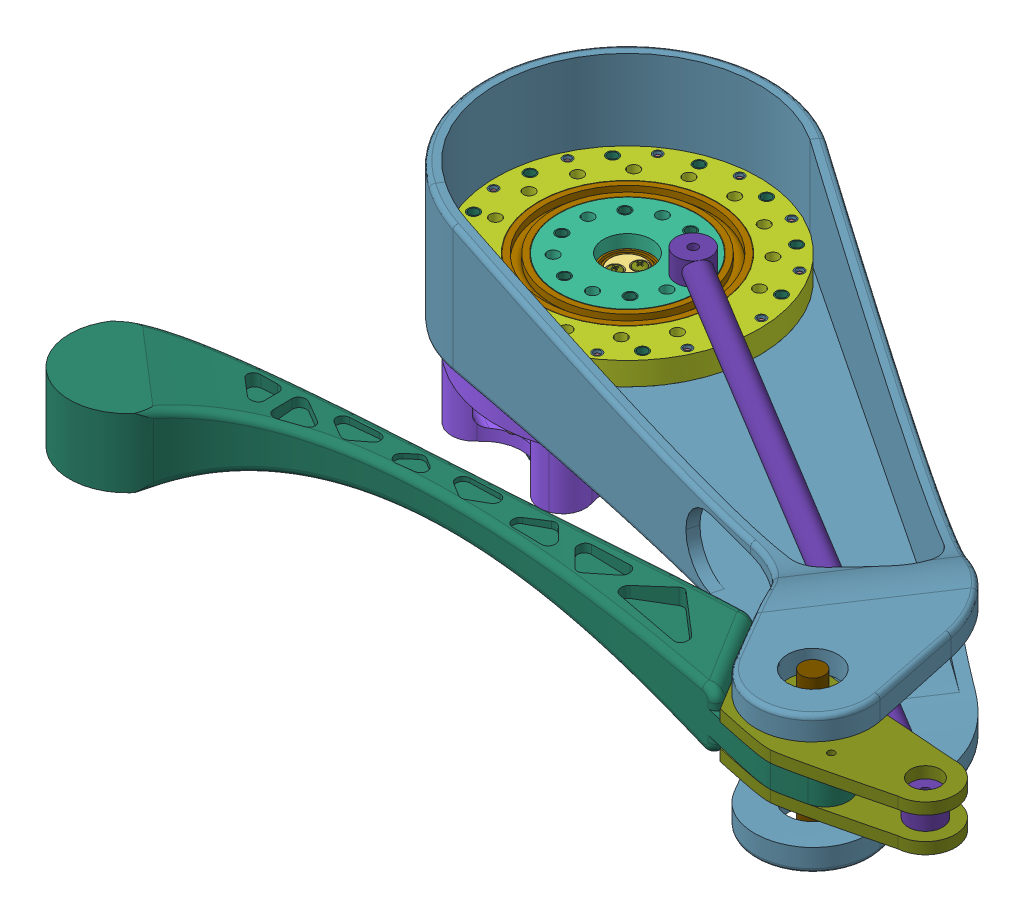
SolidWorks assembly Leg, configuration Default. Lengths in mm.
Overall size (396.87 118.19 320.81).
400 component instances, 99 part files, 9 mates.
Components (placement in the parent):
- Cycloidal-1: Cycloidal [Default] at (-40.1687 29.4235 207.1731) x (-0.342839 0 -0.939394) z (0.939394 0 -0.342839) size (162.63 70.39 162.63)
  - motor-X83008S.stp-1: motor-X83008S.stp [Default] at (19.7719 89.7915 55.1095) x (0.817868 0 0.575406) z (0 -1 0) size (114.7 114.7 37.62) (hidden)
    - base.stp-1: base.stp [Default] at (42.0794 12.0269 46.7342) size (91.6 91.6 15.61)
    - stator.stp-1: stator.stp [Default] at (42.0794 12.0269 33.1342) x (0.08493 -0.996387 0) z (0 0 1) size (83 83 8)
    - coil.stp-1: coil.stp [Default] at (39.5332 41.8984 37.1342) x (0.996387 0.08493 0) z (-0.08493 0.996387 0) size (4.4 10.2 10.5)
    - coil.stp-2: coil.stp [Default] at (34.3848 41.0025 37.1342) x (0.966502 0.256661 0) z (-0.256661 0.966502 0) size (4.4 10.2 10.5)
    - coil.stp-3: coil.stp [Default] at (29.4701 39.2261 37.1342) x (0.90725 0.420593 0) z (-0.420593 0.90725 0) size (4.4 10.2 10.5)
    - coil.stp-4: coil.stp [Default] at (24.9386 36.6233 37.1342) x (0.820431 0.571745 0) z (-0.571745 0.820431 0) size (4.4 10.2 10.5)
    - coil.stp-5: coil.stp [Default] at (20.9279 33.2732 37.1342) x (0.708685 0.705525 0) z (-0.705525 0.708685 0) size (4.4 10.2 10.5)
    - coil.stp-6: coil.stp [Default] at (17.5599 29.2775 37.1342) x (0.575405 0.817869 0) z (-0.817869 0.575405 0) size (4.4 10.2 10.5)
    - coil.stp-7: coil.stp [Default] at (14.9368 24.7576 37.1342) x (0.424642 0.905361 0) z (-0.905361 0.424642 0) size (4.4 10.2 10.5)
    - coil.stp-8: coil.stp [Default] at (13.1385 19.8509 37.1342) x (0.260976 0.965345 0) z (-0.965345 0.260976 0) size (4.4 10.2 10.5)
    - coil.stp-9: coil.stp [Default] at (12.2196 14.7066 37.1342) x (0.089381 0.995998 0) z (-0.995998 0.089381 0) size (4.4 10.2 10.5)
    - coil.stp-10: coil.stp [Default] at (12.2079 9.4807 37.1342) x (-0.08493 0.996387 0) z (-0.996387 -0.08493 0) size (4.4 10.2 10.5)
    - coil.stp-11: coil.stp [Default] at (13.1039 4.3323 37.1342) x (-0.256661 0.966502 0) z (-0.966502 -0.256661 0) size (4.4 10.2 10.5)
    - coil.stp-12: coil.stp [Default] at (14.8802 -0.5824 37.1342) x (-0.420593 0.90725 0) z (-0.90725 -0.420593 0) size (4.4 10.2 10.5)
    - coil.stp-13: coil.stp [Default] at (17.483 -5.1139 37.1342) x (-0.571745 0.820431 0) z (-0.820431 -0.571745 0) size (4.4 10.2 10.5)
    - coil.stp-14: coil.stp [Default] at (20.8332 -9.1246 37.1342) x (-0.705525 0.708685 0) z (-0.708685 -0.705525 0) size (4.4 10.2 10.5)
    - coil.stp-15: coil.stp [Default] at (24.8289 -12.4926 37.1342) x (-0.817869 0.575405 0) z (-0.575405 -0.817869 0) size (4.4 10.2 10.5)
    - coil.stp-16: coil.stp [Default] at (29.3487 -15.1157 37.1342) x (-0.905361 0.424642 0) z (-0.424642 -0.905361 0) size (4.4 10.2 10.5)
    - coil.stp-17: coil.stp [Default] at (34.2554 -16.914 37.1342) x (-0.965345 0.260976 0) z (-0.260976 -0.965345 0) size (4.4 10.2 10.5)
    - coil.stp-18: coil.stp [Default] at (39.3998 -17.8329 37.1342) x (-0.995998 0.089381 0) z (-0.089381 -0.995998 0) size (4.4 10.2 10.5)
    - coil.stp-19: coil.stp [Default] at (44.6256 -17.8446 37.1342) x (-0.996387 -0.08493 0) z (0.08493 -0.996387 0) size (4.4 10.2 10.5)
    - coil.stp-20: coil.stp [Default] at (49.7741 -16.9486 37.1342) x (-0.966502 -0.256661 0) z (0.256661 -0.966502 0) size (4.4 10.2 10.5)
    - coil.stp-21: coil.stp [Default] at (54.6887 -15.1723 37.1342) x (-0.90725 -0.420593 0) z (0.420593 -0.90725 0) size (4.4 10.2 10.5)
    - coil.stp-22: coil.stp [Default] at (59.2202 -12.5695 37.1342) x (-0.820431 -0.571745 0) z (0.571745 -0.820431 0) size (4.4 10.2 10.5)
    - coil.stp-23: coil.stp [Default] at (63.2309 -9.2193 37.1342) x (-0.708685 -0.705525 0) z (0.705525 -0.708685 0) size (4.4 10.2 10.5)
    - coil.stp-24: coil.stp [Default] at (66.599 -5.2236 37.1342) x (-0.575405 -0.817869 0) z (0.817869 -0.575405 0) size (4.4 10.2 10.5)
    - coil.stp-25: coil.stp [Default] at (69.222 -0.7038 37.1342) x (-0.424642 -0.905361 0) z (0.905361 -0.424642 0) size (4.4 10.2 10.5)
    - coil.stp-26: coil.stp [Default] at (71.0203 4.2029 37.1342) x (-0.260976 -0.965345 0) z (0.965345 -0.260976 0) size (4.4 10.2 10.5)
    - coil.stp-27: coil.stp [Default] at (71.9392 9.3473 37.1342) x (-0.089381 -0.995998 0) z (0.995998 -0.089381 0) size (4.4 10.2 10.5)
    - coil.stp-28: coil.stp [Default] at (71.9509 14.5731 37.1342) x (0.08493 -0.996387 0) z (0.996387 0.08493 0) size (4.4 10.2 10.5)
    - coil.stp-29: coil.stp [Default] at (71.055 19.7216 37.1342) x (0.256661 -0.966502 0) z (0.966502 0.256661 0) size (4.4 10.2 10.5)
    - coil.stp-30: coil.stp [Default] at (69.2786 24.6362 37.1342) x (0.420593 -0.90725 0) z (0.90725 0.420593 0) size (4.4 10.2 10.5)
    - coil.stp-31: coil.stp [Default] at (66.6758 29.1677 37.1342) x (0.571745 -0.820431 0) z (0.820431 0.571745 0) size (4.4 10.2 10.5)
    - coil.stp-32: coil.stp [Default] at (63.3257 33.1785 37.1342) x (0.705525 -0.708685 0) z (0.708685 0.705525 0) size (4.4 10.2 10.5)
    - coil.stp-33: coil.stp [Default] at (59.33 36.5465 37.1342) x (0.817869 -0.575405 0) z (0.575405 0.817869 0) size (4.4 10.2 10.5)
    - coil.stp-34: coil.stp [Default] at (54.8101 39.1695 37.1342) x (0.905361 -0.424642 0) z (0.424642 0.905361 0) size (4.4 10.2 10.5)
    - coil.stp-35: coil.stp [Default] at (49.9034 40.9678 37.1342) x (0.965345 -0.260976 0) z (0.260976 0.965345 0) size (4.4 10.2 10.5)
    - coil.stp-36: coil.stp [Default] at (44.759 41.8868 37.1342) x (0.995998 -0.089381 0) z (0.089381 0.995998 0) size (4.4 10.2 10.5)
    - rotor.stp-1: rotor.stp [Default] at (42.0794 12.0269 42.1342) x (-0.293442 0.955977 0) z (0 0 -1) size (91.8 91.8 12)
    - outrunner.stp-1: outrunner.stp [Default] at (42.0794 12.0269 30.1342) x (-0.254711 0.967017 0) z (-0.967017 -0.254711 0) size (91.8 17.01 91.8)
    - screw-mount.stp-1: screw-mount.stp [Default] at (38.1314 27.0157 27.1342) x (1 0 0) z (0 0 -1) size (7 7 6.5)
    - screw-mount.stp-2: screw-mount.stp [Default] at (27.0906 8.0789 27.1342) x (1 0 0) z (0 0 -1) size (7 7 6.5)
    - screw-mount.stp-3: screw-mount.stp [Default] at (57.0682 15.9749 27.1342) x (1 0 0) z (0 0 -1) size (7 7 6.5)
    - screw-mount.stp-4: screw-mount.stp [Default] at (46.0274 -2.9618 27.1342) x (1 0 0) z (0 0 -1) size (7 7 6.5)
    - 6702ZZ-bearing-15x21x4.stp-1: 6702ZZ-bearing-15x21x4.stp [Default] at (42.0794 12.0269 43.7342) x (1 0 0) z (0 -1 0) size (21 4 21)
    - 6702ZZ-bearing-15x21x4.stp-2: 6702ZZ-bearing-15x21x4.stp [Default] at (42.0794 12.0269 35.1342) x (1 0 0) z (0 1 0) size (21 4 21)
    - shaft.stp-1: shaft.stp [Default] at (42.0794 12.0269 20.1342) size (16 16 31.6)
    - fix-screw.stp-1: fix-screw.stp [Default] at (42.0794 12.0269 51.7342) x (1 0 0) z (0 0 -1) size (19.67 18.96 12.02)
  - Base_Plate-1: Base_Plate [Default] at (47.267 69.6573 89.1587) x (-0.64433 0 -0.764747) z (0.764747 0 -0.64433) size (40 7 40)
  - Eccentric_Shaft-1: Eccentric_Shaft [Default] at (62.181 70.3165 95.0179) x (-0.764747 0 0.64433) z (-0.64433 0 -0.764747) size (20 15 17)
    - Eccentric_Shaft_bot-1: Eccentric_Shaft_bot [Default] at (7.6302 6.3409 14.0904) size (17 5 17)
    - Eccentric_Shaft_bot-2: Eccentric_Shaft_bot [Default] at (7.6302 11.3409 14.0904) x (-1 0 0) z (0 0 -1) size (17 5 17)
    - Eccentric_Shaft_top-1: Eccentric_Shaft_top [Default] at (7.6302 16.3409 14.0904) x (-1 0 0) z (0 0 -1) size (17 5 17)
  - Cycloidal_Discs-1: Cycloidal_Discs [Default] at (46.1199 86.6573 90.1252) x (0.999784 0 -0.020763) z (-0.020763 0 -0.999784) size (79.25 5 79.73)
  - Cycloidal_Discs-2: Cycloidal_Discs [Default] at (48.4141 76.6573 88.1922) x (0.979859 0 0.19969) z (-0.19969 0 0.979859) size (79.25 5 79.73)
  - Ring_Pin_Housing-1: Ring_Pin_Housing [Default] at (47.267 76.6573 89.1587) x (0.707107 0 -0.707107) z (0.707107 0 0.707107) size (115 10.6 115)
  - Output_Shaft-1: Output_Shaft [Default] at (47.267 87.2573 89.1587) x (-0.998587 0 -0.053142) z (0.053142 0 -0.998587) size (60 10 60)
  - Cover-1: Cover [Default] at (47.267 87.2573 89.1587) x (0.707107 0 -0.707107) z (0.707107 0 0.707107) size (115 10.4 115)
  - Motor_Cover-2: Motor_Cover [Default] at (47.267 36.0573 89.1587) size (115 33.6 115)
  - radial ball bearing_68_iso-39: radial ball bearing_68_iso [ISO 15 RBB - 1860 - 32,SI,NC,32_68] at (47.267 92.2573 89.1587) x (0 1 0) z (0 0 1) size (10 78 78)
  - radial ball bearing_68_iso-40: radial ball bearing_68_iso [ISO 15 RBB - 1840 - 32,SI,NC,32_68] at (47.267 72.9573 89.1587) x (0 1 0) z (0.001003 0 0.999999) size (7 52 52)
  - Base_plate_2-1: Base_plate_2 [Default] at (47.267 69.6573 89.1587) x (0.707107 0 -0.707107) z (0.707107 0 0.707107) size (115 7 115)
  - m13_bearing-31: m13_bearing [Default] at (-10.7414 95.4081 67.0593) x (0.227678 0 0.973736) z (0.973736 0 -0.227678) size (13 16 13)
    - m6-1: m6 [Default] at (8.4921 2.5508 14.8914) size (6 16 6)
    - radial ball bearing_68_iso-1: radial ball bearing_68_iso [ISO 15 RBB - 286 - 10,SI,NC,10_68] at (8.4921 16.0508 14.8914) x (0 1 0) z (0 0 1) size (5 13 13)
    - radial ball bearing_68_iso-2: radial ball bearing_68_iso [ISO 15 RBB - 286 - 10,SI,NC,10_68] at (8.4921 11.0508 14.8914) x (0 1 0) z (0 0 1) size (5 13 13)
  - m13_bearing-32: m13_bearing [Default] at (-14.1668 95.4081 84.2801) x (0.227678 0 0.973736) z (0.973736 0 -0.227678) size (13 16 13)
    - m6-1: m6 [Default] at (8.4921 2.5508 14.8914) size (6 16 6)
    - radial ball bearing_68_iso-1: radial ball bearing_68_iso [ISO 15 RBB - 286 - 10,SI,NC,10_68] at (8.4921 16.0508 14.8914) x (0 1 0) z (0 0 1) size (5 13 13)
    - radial ball bearing_68_iso-2: radial ball bearing_68_iso [ISO 15 RBB - 286 - 10,SI,NC,10_68] at (8.4921 11.0508 14.8914) x (0 1 0) z (0 0 1) size (5 13 13)
  - m13_bearing-34: m13_bearing [Default] at (13.6125 95.5581 125.8547) x (0.227678 0 0.973736) z (0.973736 0 -0.227678) size (13 16 13)
    - m6-1: m6 [Default] at (8.4921 2.5508 14.8914) size (6 16 6)
    - radial ball bearing_68_iso-1: radial ball bearing_68_iso [ISO 15 RBB - 286 - 10,SI,NC,10_68] at (8.4921 16.0508 14.8914) x (0 1 0) z (0 0 1) size (5 13 13)
    - radial ball bearing_68_iso-2: radial ball bearing_68_iso [ISO 15 RBB - 286 - 10,SI,NC,10_68] at (8.4921 11.0508 14.8914) x (0 1 0) z (0 0 1) size (5 13 13)
  - m13_bearing-35: m13_bearing [Default] at (-0.9866 95.4081 116.0999) x (0.227678 0 0.973736) z (0.973736 0 -0.227678) size (13 16 13)
    - m6-1: m6 [Default] at (8.4921 2.5508 14.8914) size (6 16 6)
    - radial ball bearing_68_iso-1: radial ball bearing_68_iso [ISO 15 RBB - 286 - 10,SI,NC,10_68] at (8.4921 16.0508 14.8914) x (0 1 0) z (0 0 1) size (5 13 13)
    - radial ball bearing_68_iso-2: radial ball bearing_68_iso [ISO 15 RBB - 286 - 10,SI,NC,10_68] at (8.4921 11.0508 14.8914) x (0 1 0) z (0 0 1) size (5 13 13)
  - m13_bearing-36: m13_bearing [Default] at (-10.7414 95.5581 101.5009) x (0.227678 0 0.973736) z (0.973736 0 -0.227678) size (13 16 13)
    - m6-1: m6 [Default] at (8.4921 2.5508 14.8914) size (6 16 6)
    - radial ball bearing_68_iso-1: radial ball bearing_68_iso [ISO 15 RBB - 286 - 10,SI,NC,10_68] at (8.4921 16.0508 14.8914) x (0 1 0) z (0 0 1) size (5 13 13)
    - radial ball bearing_68_iso-2: radial ball bearing_68_iso [ISO 15 RBB - 286 - 10,SI,NC,10_68] at (8.4921 11.0508 14.8914) x (0 1 0) z (0 0 1) size (5 13 13)
  - m13_bearing-1: m13_bearing [Default] at (-0.8801 95.4081 62.5627) x (0.736525 0 0.676411) z (0.676411 0 -0.736525) size (13 16 13)
    - m6-1: m6 [Default] at (8.4921 2.5508 14.8914) size (6 16 6)
    - radial ball bearing_68_iso-1: radial ball bearing_68_iso [ISO 15 RBB - 286 - 10,SI,NC,10_68] at (8.4921 16.0508 14.8914) x (0 1 0) z (0 0 1) size (5 13 13)
    - radial ball bearing_68_iso-2: radial ball bearing_68_iso [ISO 15 RBB - 286 - 10,SI,NC,10_68] at (8.4921 11.0508 14.8914) x (0 1 0) z (0 0 1) size (5 13 13)
  - m13_bearing-2: m13_bearing [Default] at (48.6831 95.4081 124.0939) x (0.120271 0 0.992741) z (0.992741 0 -0.120271) size (13 16 13)
    - m6-1: m6 [Default] at (8.4921 2.5508 14.8914) size (6 16 6)
    - radial ball bearing_68_iso-1: radial ball bearing_68_iso [ISO 15 RBB - 286 - 10,SI,NC,10_68] at (8.4921 16.0508 14.8914) x (0 1 0) z (0 0 1) size (5 13 13)
    - radial ball bearing_68_iso-2: radial ball bearing_68_iso [ISO 15 RBB - 286 - 10,SI,NC,10_68] at (8.4921 11.0508 14.8914) x (0 1 0) z (0 0 1) size (5 13 13)
  - m13_bearing-3: m13_bearing [Default] at (32.7832 95.4081 34.9886) x (-0.046141 0 0.998935) z (0.998935 0 0.046141) size (13 16 13)
    - m6-1: m6 [Default] at (8.4921 2.5508 14.8914) size (6 16 6)
    - radial ball bearing_68_iso-1: radial ball bearing_68_iso [ISO 15 RBB - 286 - 10,SI,NC,10_68] at (8.4921 16.0508 14.8914) x (0 1 0) z (0 0 1) size (5 13 13)
    - radial ball bearing_68_iso-2: radial ball bearing_68_iso [ISO 15 RBB - 286 - 10,SI,NC,10_68] at (8.4921 11.0508 14.8914) x (0 1 0) z (0 0 1) size (5 13 13)
  - m13_bearing-4: m13_bearing [Default] at (77.1902 95.4081 81.0003) x (0.022268 0 0.999752) z (0.999752 0 -0.022268) size (13 16 13)
    - m6-1: m6 [Default] at (8.4921 2.5508 14.8914) size (6 16 6)
    - radial ball bearing_68_iso-1: radial ball bearing_68_iso [ISO 15 RBB - 286 - 10,SI,NC,10_68] at (8.4921 16.0508 14.8914) x (0 1 0) z (0 0 1) size (5 13 13)
    - radial ball bearing_68_iso-2: radial ball bearing_68_iso [ISO 15 RBB - 286 - 10,SI,NC,10_68] at (8.4921 11.0508 14.8914) x (0 1 0) z (0 0 1) size (5 13 13)
  - m13_bearing-5: m13_bearing [Default] at (73.474 95.4081 98.7828) x (0.059133 0 0.99825) z (0.99825 0 -0.059133) size (13 16 13)
    - m6-1: m6 [Default] at (8.4921 2.5508 14.8914) size (6 16 6)
    - radial ball bearing_68_iso-1: radial ball bearing_68_iso [ISO 15 RBB - 286 - 10,SI,NC,10_68] at (8.4921 16.0508 14.8914) x (0 1 0) z (0 0 1) size (5 13 13)
    - radial ball bearing_68_iso-2: radial ball bearing_68_iso [ISO 15 RBB - 286 - 10,SI,NC,10_68] at (8.4921 11.0508 14.8914) x (0 1 0) z (0 0 1) size (5 13 13)
  - m13_bearing-6: m13_bearing [Default] at (12.9248 95.4081 46.7315) x (0.451561 0 0.89224) z (0.89224 0 -0.451561) size (13 16 13)
    - m6-1: m6 [Default] at (8.4921 2.5508 14.8914) size (6 16 6)
    - radial ball bearing_68_iso-1: radial ball bearing_68_iso [ISO 15 RBB - 286 - 10,SI,NC,10_68] at (8.4921 16.0508 14.8914) x (0 1 0) z (0 0 1) size (5 13 13)
    - radial ball bearing_68_iso-2: radial ball bearing_68_iso [ISO 15 RBB - 286 - 10,SI,NC,10_68] at (8.4921 11.0508 14.8914) x (0 1 0) z (0 0 1) size (5 13 13)
  - m13_bearing-7: m13_bearing [Default] at (56.6452 95.4081 32.3406) x (-0.545813 0 0.837907) z (0.837907 0 0.545813) size (13 16 13)
    - m6-1: m6 [Default] at (8.4921 2.5508 14.8914) size (6 16 6)
    - radial ball bearing_68_iso-1: radial ball bearing_68_iso [ISO 15 RBB - 286 - 10,SI,NC,10_68] at (8.4921 16.0508 14.8914) x (0 1 0) z (0 0 1) size (5 13 13)
    - radial ball bearing_68_iso-2: radial ball bearing_68_iso [ISO 15 RBB - 286 - 10,SI,NC,10_68] at (8.4921 11.0508 14.8914) x (0 1 0) z (0 0 1) size (5 13 13)
  - m13_bearing-8: m13_bearing [Default] at (63.0373 95.4081 51.3153) x (0.158553 0 0.98735) z (0.98735 0 -0.158553) size (13 16 13)
    - m6-1: m6 [Default] at (8.4921 2.5508 14.8914) size (6 16 6)
    - radial ball bearing_68_iso-1: radial ball bearing_68_iso [ISO 15 RBB - 286 - 10,SI,NC,10_68] at (8.4921 16.0508 14.8914) x (0 1 0) z (0 0 1) size (5 13 13)
    - radial ball bearing_68_iso-2: radial ball bearing_68_iso [ISO 15 RBB - 286 - 10,SI,NC,10_68] at (8.4921 11.0508 14.8914) x (0 1 0) z (0 0 1) size (5 13 13)
  - m13_bearing-9: m13_bearing [Default] at (83.8577 95.4081 55.5358) x (-0.687134 0 0.72653) z (0.72653 0 0.687134) size (13 16 13)
    - m6-1: m6 [Default] at (8.4921 2.5508 14.8914) size (6 16 6)
    - radial ball bearing_68_iso-1: radial ball bearing_68_iso [ISO 15 RBB - 286 - 10,SI,NC,10_68] at (8.4921 16.0508 14.8914) x (0 1 0) z (0 0 1) size (5 13 13)
    - radial ball bearing_68_iso-2: radial ball bearing_68_iso [ISO 15 RBB - 286 - 10,SI,NC,10_68] at (8.4921 11.0508 14.8914) x (0 1 0) z (0 0 1) size (5 13 13)
  - m13_bearing-11: m13_bearing [Default] at (30.1977 95.4081 135.7424) x (0.57351 0 0.819198) z (0.819198 0 -0.57351) size (13 16 13)
    - m6-1: m6 [Default] at (8.4921 2.5508 14.8914) size (6 16 6)
    - radial ball bearing_68_iso-1: radial ball bearing_68_iso [ISO 15 RBB - 286 - 10,SI,NC,10_68] at (8.4921 16.0508 14.8914) x (0 1 0) z (0 0 1) size (5 13 13)
    - radial ball bearing_68_iso-2: radial ball bearing_68_iso [ISO 15 RBB - 286 - 10,SI,NC,10_68] at (8.4921 11.0508 14.8914) x (0 1 0) z (0 0 1) size (5 13 13)
  - m13_bearing-12: m13_bearing [Default] at (62.8861 95.4081 115.3744) x (0.184178 0 0.982893) z (0.982893 0 -0.184178) size (13 16 13)
    - m6-1: m6 [Default] at (8.4921 2.5508 14.8914) size (6 16 6)
    - radial ball bearing_68_iso-1: radial ball bearing_68_iso [ISO 15 RBB - 286 - 10,SI,NC,10_68] at (8.4921 16.0508 14.8914) x (0 1 0) z (0 0 1) size (5 13 13)
    - radial ball bearing_68_iso-2: radial ball bearing_68_iso [ISO 15 RBB - 286 - 10,SI,NC,10_68] at (8.4921 11.0508 14.8914) x (0 1 0) z (0 0 1) size (5 13 13)
  - socket button head screw_iso-2: socket button head screw_iso [ISO 7380 - M4 x 12 - 12N] at (47.267 67.4573 134.1587) x (0 1 0) z (-0.724148 0 0.689645) size (14.2 7.6 7.6)
  - socket button head screw_iso-3: socket button head screw_iso [ISO 7380 - M4 x 12 - 12N] at (15.4472 67.4573 57.3389) x (0 1 0) z (-0.724148 0 0.689645) size (14.2 7.6 7.6)
  - socket button head screw_iso-4: socket button head screw_iso [ISO 7380 - M4 x 12 - 12N] at (30.0462 67.4573 47.5841) x (0 1 0) z (-0.724148 0 0.689645) size (14.2 7.6 7.6)
  - socket button head screw_iso-5: socket button head screw_iso [ISO 7380 - M4 x 12 - 12N] at (47.267 67.4573 44.1587) x (0 1 0) z (-0.724148 0 0.689645) size (14.2 7.6 7.6)
  - socket button head screw_iso-6: socket button head screw_iso [ISO 7380 - M4 x 12 - 12N] at (64.4877 67.4573 47.5841) x (0 1 0) z (-0.724148 0 0.689645) size (14.2 7.6 7.6)
  - socket button head screw_iso-8: socket button head screw_iso [ISO 7380 - M4 x 12 - 12N] at (88.8416 67.4573 71.9379) x (0 1 0) z (-0.724148 0 0.689645) size (14.2 7.6 7.6)
  - socket button head screw_iso-9: socket button head screw_iso [ISO 7380 - M4 x 12 - 12N] at (92.267 67.4573 89.1587) x (0 1 0) z (-0.724148 0 0.689645) size (14.2 7.6 7.6)
  - socket button head screw_iso-10: socket button head screw_iso [ISO 7380 - M4 x 12 - 12N] at (88.8416 67.4573 106.3794) x (0 1 0) z (-0.724148 0 0.689645) size (14.2 7.6 7.6)
  - socket button head screw_iso-11: socket button head screw_iso [ISO 7380 - M4 x 12 - 12N] at (79.0868 67.4573 120.9785) x (0 1 0) z (-0.724148 0 0.689645) size (14.2 7.6 7.6)
  - M3x35-6: M3x35 [Default] at (9.0832 59.8573 50.9749) size (6 36.2 6)
  - M3x35-7: M3x35 [Default] at (-4.893 59.8573 75.1824) size (6 36.2 6)
  - M3x35-8: M3x35 [Default] at (-4.893 59.8573 103.1349) size (6 36.2 6)
  - M3x35-9: M3x35 [Default] at (9.0832 59.8573 127.3424) size (6 36.2 6)
  - M3x35-10: M3x35 [Default] at (33.2908 59.8573 141.3187) size (6 36.2 6)
  - M3x35-11: M3x35 [Default] at (61.2432 59.8573 141.3187) size (6 36.2 6)
  - M3x35-12: M3x35 [Default] at (85.4508 59.8573 127.3424) size (6 36.2 6)
  - M3x35-13: M3x35 [Default] at (99.427 59.8573 103.1349) size (6 36.2 6)
  - M3x35-14: M3x35 [Default] at (99.427 59.8573 75.1824) size (6 36.2 6)
  - M3x35-15: M3x35 [Default] at (85.4508 59.8573 50.9749) size (6 36.2 6)
  - M3x35-16: M3x35 [Default] at (33.2908 59.8573 36.9987) size (6 36.2 6)
  - M3x35-17: M3x35 [Default] at (61.2432 59.8573 36.9987) size (6 36.2 6)
  - m13_bearing-13: m13_bearing [Default] at (21.9503 95.0081 60.165) x (0 0 1) z (1 0 0) size (13 16 13)
    - m6-1: m6 [Default] at (8.4921 2.5508 14.8914) size (6 16 6)
    - radial ball bearing_68_iso-1: radial ball bearing_68_iso [ISO 15 RBB - 286 - 10,SI,NC,10_68] at (8.4921 16.0508 14.8914) x (0 1 0) z (0 0 1) size (5 13 13)
    - radial ball bearing_68_iso-2: radial ball bearing_68_iso [ISO 15 RBB - 286 - 10,SI,NC,10_68] at (8.4921 11.0508 14.8914) x (0 1 0) z (0 0 1) size (5 13 13)
  - m13_bearing-14: m13_bearing [Default] at (31.351 95.0081 72.3113) x (-0.995553 0 0.094199) z (0.094199 0 0.995553) size (13 16 13)
    - m6-1: m6 [Default] at (8.4921 2.5508 14.8914) size (6 16 6)
    - radial ball bearing_68_iso-1: radial ball bearing_68_iso [ISO 15 RBB - 286 - 10,SI,NC,10_68] at (8.4921 16.0508 14.8914) x (0 1 0) z (0 0 1) size (5 13 13)
    - radial ball bearing_68_iso-2: radial ball bearing_68_iso [ISO 15 RBB - 286 - 10,SI,NC,10_68] at (8.4921 11.0508 14.8914) x (0 1 0) z (0 0 1) size (5 13 13)
  - m13_bearing-15: m13_bearing [Default] at (19.8333 95.0081 99.9459) x (0 0 1) z (1 0 0) size (13 16 13)
    - m6-1: m6 [Default] at (8.4921 2.5508 14.8914) size (6 16 6)
    - radial ball bearing_68_iso-1: radial ball bearing_68_iso [ISO 15 RBB - 286 - 10,SI,NC,10_68] at (8.4921 16.0508 14.8914) x (0 1 0) z (0 0 1) size (5 13 13)
    - radial ball bearing_68_iso-2: radial ball bearing_68_iso [ISO 15 RBB - 286 - 10,SI,NC,10_68] at (8.4921 11.0508 14.8914) x (0 1 0) z (0 0 1) size (5 13 13)
  - m13_bearing-16: m13_bearing [Default] at (60.3496 95.0081 87.0135) x (0.852631 0 -0.522513) z (-0.522513 0 -0.852631) size (13 16 13)
    - m6-1: m6 [Default] at (8.4921 2.5508 14.8914) size (6 16 6)
    - radial ball bearing_68_iso-1: radial ball bearing_68_iso [ISO 15 RBB - 286 - 10,SI,NC,10_68] at (8.4921 16.0508 14.8914) x (0 1 0) z (0 0 1) size (5 13 13)
    - radial ball bearing_68_iso-2: radial ball bearing_68_iso [ISO 15 RBB - 286 - 10,SI,NC,10_68] at (8.4921 11.0508 14.8914) x (0 1 0) z (0 0 1) size (5 13 13)
  - m13_bearing-17: m13_bearing [Default] at (45.2305 95.0081 121.432) x (0.95663 0 0.291306) z (0.291306 0 -0.95663) size (13 16 13)
    - m6-1: m6 [Default] at (8.4921 2.5508 14.8914) size (6 16 6)
    - radial ball bearing_68_iso-1: radial ball bearing_68_iso [ISO 15 RBB - 286 - 10,SI,NC,10_68] at (8.4921 16.0508 14.8914) x (0 1 0) z (0 0 1) size (5 13 13)
    - radial ball bearing_68_iso-2: radial ball bearing_68_iso [ISO 15 RBB - 286 - 10,SI,NC,10_68] at (8.4921 11.0508 14.8914) x (0 1 0) z (0 0 1) size (5 13 13)
  - m13_bearing-18: m13_bearing [Default] at (55.3431 95.0081 81.8889) x (0 0 1) z (1 0 0) size (13 16 13)
    - m6-1: m6 [Default] at (8.4921 2.5508 14.8914) size (6 16 6)
    - radial ball bearing_68_iso-1: radial ball bearing_68_iso [ISO 15 RBB - 286 - 10,SI,NC,10_68] at (8.4921 16.0508 14.8914) x (0 1 0) z (0 0 1) size (5 13 13)
    - radial ball bearing_68_iso-2: radial ball bearing_68_iso [ISO 15 RBB - 286 - 10,SI,NC,10_68] at (8.4921 11.0508 14.8914) x (0 1 0) z (0 0 1) size (5 13 13)
  - M3x4x4.2_brass_insert-1: M3x4x4.2_brass_insert [Default] at (-4.893 93.2573 75.1824) x (0.984609 0 -0.174769) z (0.174769 0 0.984609) size (4 4 4)
  - M3x4x4.2_brass_insert-2: M3x4x4.2_brass_insert [Default] at (9.0832 97.2573 50.9749) x (-0.680278 0 -0.732954) z (-0.732954 0 0.680278) size (4 4 4)
  - M3x4x4.2_brass_insert-3: M3x4x4.2_brass_insert [Default] at (33.2908 97.2573 36.9987) x (-0.509546 0 -0.860444) z (-0.860444 0 0.509546) size (4 4 4)
  - M3x4x4.2_brass_insert-6: M3x4x4.2_brass_insert [Default] at (99.427 97.2573 75.1824) x (-0.680278 0 -0.732954) z (-0.732954 0 0.680278) size (4 4 4)
  - M3x4x4.2_brass_insert-8: M3x4x4.2_brass_insert [Default] at (85.4508 93.2573 127.3424) x (-0.970393 0 0.241533) z (-0.241533 0 -0.970393) size (4 4 4)
  - M3x4x4.2_brass_insert-14: M3x4x4.2_brass_insert [Default] at (61.2432 97.2573 36.9987) x (0.509546 0 0.860444) z (0.860444 0 -0.509546) size (4 4 4)
  - M3x4x4.2_brass_insert-15: M3x4x4.2_brass_insert [Default] at (85.4508 93.2573 50.9749) x (0.897191 0 -0.441644) z (0.441644 0 0.897191) size (4 4 4)
  - M3x4x4.2_brass_insert-16: M3x4x4.2_brass_insert [Default] at (99.427 97.2573 103.1349) x (-0.680278 0 -0.732954) z (-0.732954 0 0.680278) size (4 4 4)
  - M3x4x4.2_brass_insert-17: M3x4x4.2_brass_insert [Default] at (61.2432 97.2573 141.3187) x (0.680278 0 0.732954) z (0.732954 0 -0.680278) size (4 4 4)
  - M3x4x4.2_brass_insert-19: M3x4x4.2_brass_insert [Default] at (33.2908 97.2573 141.3187) x (0.680278 0 0.732954) z (0.732954 0 -0.680278) size (4 4 4)
  - M3x4x4.2_brass_insert-20: M3x4x4.2_brass_insert [Default] at (9.0832 97.2573 127.3424) x (0.680278 0 0.732954) z (0.732954 0 -0.680278) size (4 4 4)
  - M3x4x4.2_brass_insert-21: M3x4x4.2_brass_insert [Default] at (-4.893 97.2573 103.1349) x (0.680278 0 0.732954) z (0.732954 0 -0.680278) size (4 4 4)
  - M4x6x5.5_brass_insert-47: M4x6x5.5_brass_insert [Default] at (5.6924 92.8573 71.9379) x (0.474598 0 0.880203) z (0 1 0) size (5 5 6)
  - M4x6x5.5_brass_insert-48: M4x6x5.5_brass_insert [Default] at (2.267 92.8573 89.1587) x (0.260051 0 0.965595) z (0 1 0) size (5 5 6)
  - M4x6x5.5_brass_insert-49: M4x6x5.5_brass_insert [Default] at (5.6924 87.0073 106.3794) x (-0.745833 0 0.666133) z (0 -1 0) size (5 5 6)
  - M4x6x5.5_brass_insert-50: M4x6x5.5_brass_insert [Default] at (15.4472 86.8573 120.9785) x (-0.745833 0 0.666133) z (0 -1 0) size (5 5 6)
  - M4x6x5.5_brass_insert-51: M4x6x5.5_brass_insert [Default] at (30.0462 87.0073 130.7332) x (0.260051 0 -0.965595) z (0 -1 0) size (5 5 6)
  - M4x6x5.5_brass_insert-1: M4x6x5.5_brass_insert [Default] at (36.8417 86.4573 68.6571) x (-0.745833 0 0.666133) z (0 -1 0) size (5 5 6)
  - M4x6x5.5_brass_insert-4: M4x6x5.5_brass_insert [Default] at (70.2345 92.4573 90.3809) x (0.260051 0 0.965595) z (0 1 0) size (5 5 6)
  - M4x6x5.5_brass_insert-5: M4x6x5.5_brass_insert [Default] at (57.6922 92.4573 109.6602) x (0.260051 0 0.965595) z (0 1 0) size (5 5 6)
  - M4x6x5.5_brass_insert-6: M4x6x5.5_brass_insert [Default] at (34.7247 92.4573 108.438) x (0.260051 0 0.965595) z (0 1 0) size (5 5 6)
  - M4x6x5.5_brass_insert-7: M4x6x5.5_brass_insert [Default] at (24.2995 92.4573 87.9364) x (0.175665 0 0.98445) z (0 1 0) size (5 5 6)
  - M4x6x5.5_brass_insert-8: M4x6x5.5_brass_insert [Default] at (48.4892 97.2573 66.1912) x (0.260051 0 0.965595) z (0 1 0) size (5 5 6)
  - M4x6x5.5_brass_insert-9: M4x6x5.5_brass_insert [Default] at (27.9877 97.2573 76.6164) x (0.260051 0 0.965595) z (0 1 0) size (5 5 6)
  - M4x6x5.5_brass_insert-10: M4x6x5.5_brass_insert [Default] at (26.7654 97.2573 99.5839) x (0.260051 0 0.965595) z (0 1 0) size (5 5 6)
  - M4x6x5.5_brass_insert-11: M4x6x5.5_brass_insert [Default] at (46.0447 97.2573 112.1262) x (0.260051 0 0.965595) z (0 1 0) size (5 5 6)
  - M4x6x5.5_brass_insert-13: M4x6x5.5_brass_insert [Default] at (66.5463 97.2573 101.7009) x (0.260051 0 0.965595) z (0 1 0) size (5 5 6)
  - M4x6x5.5_brass_insert-14: M4x6x5.5_brass_insert [Default] at (67.7686 97.2573 78.7334) x (0.260051 0 0.965595) z (0 1 0) size (5 5 6)
  - M4x6x5.5_brass_insert-15: M4x6x5.5_brass_insert [Default] at (59.8092 92.4573 69.8794) x (0.151918 0 0.988393) z (0 1 0) size (5 5 6)
  - M4x6x5.5_brass_insert-20: M4x6x5.5_brass_insert [Default] at (64.4877 86.8573 130.7332) x (-0.745833 0 0.666133) z (0 -1 0) size (5 5 6)
  - M4x6x5.5_brass_insert-21: M4x6x5.5_brass_insert [Default] at (47.267 86.8573 134.1587) x (-0.745833 0 0.666133) z (0 -1 0) size (5 5 6)
  - M4x6x5.5_brass_insert-22: M4x6x5.5_brass_insert [Default] at (15.4472 86.8573 57.3389) x (0.623293 0 0.781988) z (0 -1 0) size (5 5 6)
  - M4x6x5.5_brass_insert-23: M4x6x5.5_brass_insert [Default] at (30.0462 86.8573 47.5841) x (0.623293 0 0.781988) z (0 -1 0) size (5 5 6)
  - M4x6x5.5_brass_insert-24: M4x6x5.5_brass_insert [Default] at (79.0868 86.8573 120.9785) x (0.541965 0 0.840401) z (0 -1 0) size (5 5 6)
  - M4x6x5.5_brass_insert-25: M4x6x5.5_brass_insert [Default] at (88.8416 86.8573 106.3794) x (-0.745833 0 0.666133) z (0 -1 0) size (5 5 6)
  - M4x6x5.5_brass_insert-26: M4x6x5.5_brass_insert [Default] at (92.267 86.8573 89.1587) x (-0.745833 0 0.666133) z (0 -1 0) size (5 5 6)
  - M4x6x5.5_brass_insert-27: M4x6x5.5_brass_insert [Default] at (88.8416 86.8573 71.9379) x (-0.745833 0 0.666133) z (0 -1 0) size (5 5 6)
  - M4x6x5.5_brass_insert-28: M4x6x5.5_brass_insert [Default] at (79.0868 92.8573 57.3389) x (0.260051 0 0.965595) z (0 1 0) size (5 5 6)
  - M4x6x5.5_brass_insert-29: M4x6x5.5_brass_insert [Default] at (64.4877 86.8573 47.5841) x (-0.142939 0 0.989731) z (0 -1 0) size (5 5 6)
  - M4x6x5.5_brass_insert-31: M4x6x5.5_brass_insert [Default] at (47.267 86.8573 44.1587) x (-0.220341 0 0.975423) z (0 -1 0) size (5 5 6)
  - M4x6x5.5_brass_insert-34: M4x6x5.5_brass_insert [Default] at (1.8007 97.2573 62.9087) x (0.260051 0 0.965595) z (0 1 0) size (5 5 6)
  - M4x6x5.5_brass_insert-35: M4x6x5.5_brass_insert [Default] at (-5.233 97.2573 89.1587) x (0.260051 0 0.965595) z (0 1 0) size (5 5 6)
  - M4x6x5.5_brass_insert-36: M4x6x5.5_brass_insert [Default] at (1.8007 97.2573 115.4087) x (0.260051 0 0.965595) z (0 1 0) size (5 5 6)
  - M4x6x5.5_brass_insert-37: M4x6x5.5_brass_insert [Default] at (21.017 97.2573 134.625) x (0.260051 0 0.965595) z (0 1 0) size (5 5 6)
  - M4x6x5.5_brass_insert-38: M4x6x5.5_brass_insert [Default] at (47.267 97.2573 141.6587) x (0.260051 0 0.965595) z (0 1 0) size (5 5 6)
  - M4x6x5.5_brass_insert-39: M4x6x5.5_brass_insert [Default] at (73.517 97.2573 134.625) x (0.260051 0 0.965595) z (0 1 0) size (5 5 6)
  - M4x6x5.5_brass_insert-40: M4x6x5.5_brass_insert [Default] at (92.7333 97.2573 115.4087) x (0.260051 0 0.965595) z (0 1 0) size (5 5 6)
  - M4x6x5.5_brass_insert-41: M4x6x5.5_brass_insert [Default] at (99.767 97.2573 89.1587) x (0.260051 0 0.965595) z (0 1 0) size (5 5 6)
  - M4x6x5.5_brass_insert-42: M4x6x5.5_brass_insert [Default] at (92.7333 97.2573 62.9087) x (0.260051 0 0.965595) z (0 1 0) size (5 5 6)
  - M4x6x5.5_brass_insert-43: M4x6x5.5_brass_insert [Default] at (73.517 97.2573 43.6923) x (0.260051 0 0.965595) z (0 1 0) size (5 5 6)
  - M4x6x5.5_brass_insert-44: M4x6x5.5_brass_insert [Default] at (47.267 97.2573 36.6587) x (0.260051 0 0.965595) z (0 1 0) size (5 5 6)
  - M4x6x5.5_brass_insert-45: M4x6x5.5_brass_insert [Default] at (21.017 97.2573 43.6923) x (0.260051 0 0.965595) z (0 1 0) size (5 5 6)
  - pan cross head_am-1: pan cross head_am [B18.6.7M - M3 x 0.5 x 20 Type I Cross Recessed PHMS --20N] at (44.6897 92.5573 86.0997) x (0 -1 0) z (0.748822 0 0.662771) size (22.37 5.6 5.6)
  - pan cross head_am-3: pan cross head_am [B18.6.7M - M3 x 0.5 x 20 Type I Cross Recessed PHMS --20N] at (49.8443 92.5573 92.2177) x (0 -1 0) z (0.940321 0 0.340288) size (22.37 5.6 5.6)
